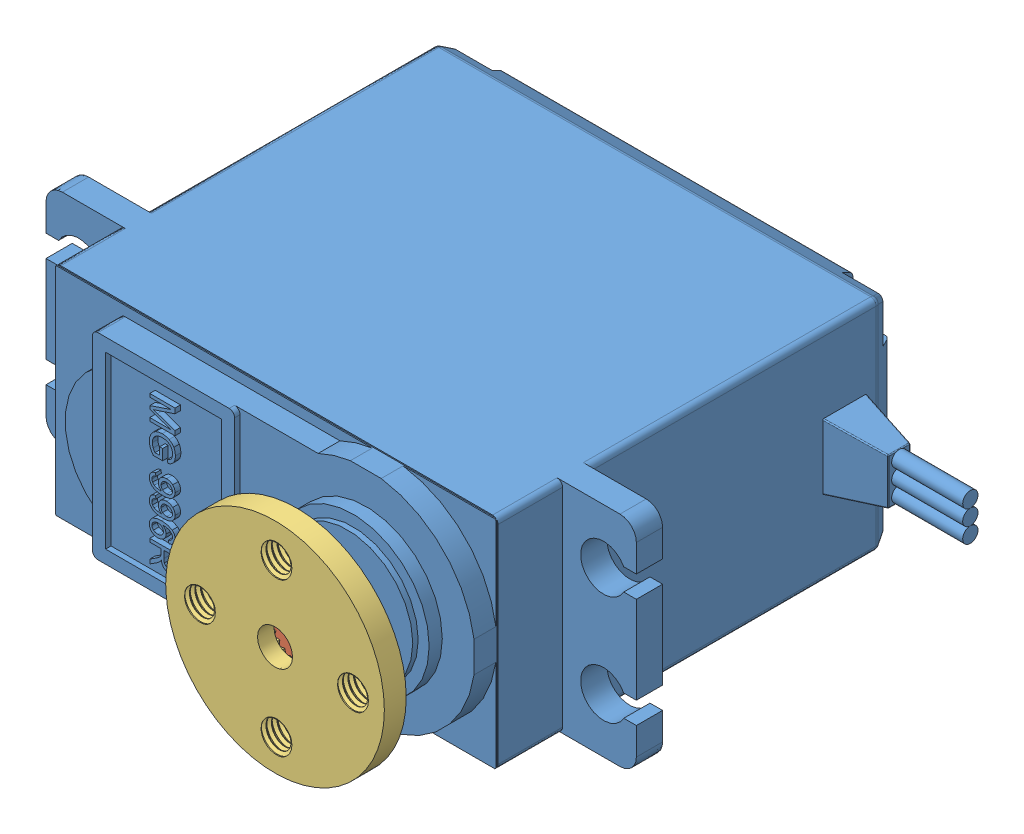
SolidWorks assembly MG996 v1 v12, configuration 預設. Lengths in mm.
Overall size (58.77 20 47.15).
4 component instances, 3 part files, 0 mates.
Components (placement in the parent):
- MG996 v1 v12(2)^MG996 v1 v12-1: MG996 v1 v12(2)^MG996 v1 v12 [預設] at origin size (58.77 20 47.15) (virtual)
  - servo body^MG996 v1 v12(2)_MG996 v1 v12-1: servo body^MG996 v1 v12(2)_MG996 v1 v12 [預設] at (-10.25 -2.0832 -1.9668) size (58.77 20 40.5) (virtual)
  - TowerPro-MG995_pulley v1^MG996 v1 v12(2)_MG996 v1 v12-1: TowerPro-MG995_pulley v1^MG996 v1 v12(2)_MG996 v1 v12 [預設] at (0 -2.0832 2.0832) x (1 0 0) z (0 -1 0) size (5.79 14 5.78) (virtual)
  - 複製 of servo dise v1^MG996 v1 v12(2)_MG996 v1 v12-1: 複製 of servo dise v1^MG996 v1 v12(2)_MG996 v1 v12 [預設] at (-10.25 -2.0832 -32.456) x (1 0 0) z (0 -1 0) size (20 5.25 20) (virtual)
